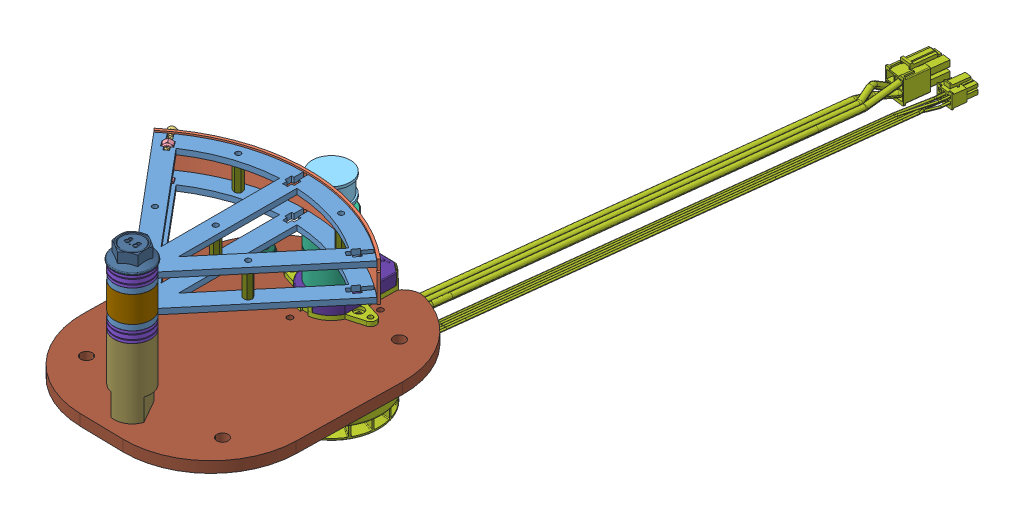
SolidWorks assembly StackedBow, configuration Default. Lengths in mm.
Overall size (130.54 146.72 171.44).
34 component instances, 25 part files, 59 mates.
Components (placement in the parent):
- BowCap-2: BowCap [Default] at origin size (128.56 3.17 110.49)
- BowCap-1: BowCap [Default] at (0 18.2 0) size (128.56 3.17 110.49)
- BowSpacer2-1: BowSpacer2 [Default] at (0 10.9625 76.6044) x (0 0 1) z (-1 0 0) size (24.99 22.7 130.54)
- 91290A053_Black-Oxide Alloy Steel Socket Head Screw-1: 91290A053_Black-Oxide Alloy Steel Socket Head Screw [91290A053] at (-56.2804 20.0625 -0.8589) x (-0.663758 -0.571718 0.482249) z (-0.587785 0 -0.809017) size (4.5 4.5 16.62)
- 94205A101_316 Stainless Steel Nylon-Insert Locknut-3: 94205A101_316 Stainless Steel Nylon-Insert Locknut [94205A101] at (-55.5457 20.0625 0.1523) x (0.809017 0 -0.587785) z (0 -1 0) size (5 3.99 5.77)
- 91290A053_Black-Oxide Alloy Steel Socket Head Screw-2: 91290A053_Black-Oxide Alloy Steel Socket Head Screw [91290A053] at (-56.2804 1.8625 -0.8589) x (-0.545652 -0.738308 0.39644) z (-0.587785 0 -0.809017) size (4.5 4.5 16.62)
- 94205A101_316 Stainless Steel Nylon-Insert Locknut-2: 94205A101_316 Stainless Steel Nylon-Insert Locknut [94205A101] at (-55.5457 1.8625 0.1523) x (0.809017 0 -0.587785) z (0 -1 0) size (5 3.99 5.77)
- Barrel-1: Barrel [Default] at (2.174 4.7125 -35.8745) x (0.993133 0 0.116992) z (-0.116992 0 0.993133) size (22 32.5 22)
- 2469K2_Clamping Shaft Coupling-1: 2469K2_Clamping Shaft Coupling [2469K2] at (2.174 -18.9188 -35.8745) x (0 1 0) z (-0.993133 0 -0.116992) size (35 24 24)
- EC60fl-200W-V2-1: EC60fl-200W-V2 [Default] at (2.174 -29.7 -35.8745) x (0 -1 0) z (-0.993133 0 -0.116992) size (68.19 353.93 60)
- 6655K55_Thrust Ball Bearing-1: 6655K55_Thrust Ball Bearing [6655K55] at (0 -3.175 76.6044) size (21 6.35 21)
- 6655K55_Thrust Ball Bearing-2: 6655K55_Thrust Ball Bearing [6655K55] at (0 24.55 76.6044) size (21 6.35 21)
- BowSpacer3-1: BowSpacer3 [Default] at (0 3.1875 76.6044) size (21 15 21)
- 94036A645_Class 8.8 Steel Flanged Hex Head Screw-1: 94036A645_Class 8.8 Steel Flanged Hex Head Screw [94036A645] at (0 27.725 76.6044) x (1 0 0) z (0 1 0) size (22.3 22.3 54.77)
- Base Plate-1: Base Plate [Default] at (1.2078 -52.8 14.1161) x (-0.019325 0 0.999813) z (-0.999813 0 -0.019325) size (158.6 6.35 125)
- ShaftMount-1: ShaftMount [Default] at (0 -46.45 76.6044) x (0.868119 0 -0.496357) z (0.496357 0 0.868119) size (21 40.1 21)
- 98952A442_Aluminum Male-Female Threaded Hex Standoff-1: 98952A442_Aluminum Male-Female Threaded Hex Standoff [98952A442] at (-37.8185 -68.8 -36.6475) x (0 1 0) z (-0.575536 0 0.817776) size (58.72 15.01 13)
- 91287A207_18-8 Stainless Steel Hex Head Screw-1: 91287A207_18-8 Stainless Steel Hex Head Screw [91287A207] at (-37.8185 -100.8 -36.6475) x (0.849418 0 0.527721) z (0 -1 0) size (10 11.55 18.36)
- 90576A115_Medium-Strength Steel Nylon-Insert Locknut-1: 90576A115_Medium-Strength Steel Nylon-Insert Locknut [90576A115] at (-37.8185 -43.45 -36.6475) x (1 0 0) z (0 1 0) size (10 11.55 6.37)
- 95947A511_Aluminum Female Threaded Hex Standoff-1: 95947A511_Aluminum Female Threaded Hex Standoff [95947A511] at (-26.8742 3.1875 36.7984) x (0 1 0) z (0 0 1) size (15.38 4.5 5.2)
- 95947A511_Aluminum Female Threaded Hex Standoff-2: 95947A511_Aluminum Female Threaded Hex Standoff [95947A511] at (-29.3566 3.1875 -13.7459) x (0 1 0) z (0.188455 0 0.982082) size (15.38 4.5 5.2)
- 95947A511_Aluminum Female Threaded Hex Standoff-3: 95947A511_Aluminum Female Threaded Hex Standoff [95947A511] at (0 3.1875 28.6044) x (0 1 0) z (0.395734 0 0.918365) size (15.38 4.5 5.2)
- 95947A511_Aluminum Female Threaded Hex Standoff-4: 95947A511_Aluminum Female Threaded Hex Standoff [95947A511] at (26.8742 3.1875 36.7984) x (0 1 0) z (0.6 0 0.8) size (15.38 4.5 5.2)
- 95947A511_Aluminum Female Threaded Hex Standoff-5: 95947A511_Aluminum Female Threaded Hex Standoff [95947A511] at (30.1914 3.1875 -13.4704) x (0 1 0) z (0.773678 0 0.63358) size (15.38 4.5 5.2)
- CUI_DEVICES_CUI_DEVICES_AMT102-0048-N8000-W-1: CUI_DEVICES_CUI_DEVICES_AMT102-0048-N8000-W [Default] at (2.174 -42.68 -35.8745) x (-0.999813 0 -0.019325) z (0 1 0) size (52.5 46.23 9.15)
  - CUI_DEVICES_AMT-102-Top-Cover-REV-I-1: CUI_DEVICES_AMT-102-Top-Cover-REV-I [Default] at (0 0 5.23) x (-1 0 0) z (0 0 -1) size (28.6 43.26 6.55)
  - CUI_DEVICES_AMT-Sleeve-REV-D(8 mm)-1: CUI_DEVICES_AMT-Sleeve-REV-D(8 mm) [Default] at (0 0 -2.42) x (0.999996 0.002864 0) z (0 0 1) size (10.79 10.79 7.8)
  - CUI_DEVICES_AMT-Hub-Top-REV-D1-1: CUI_DEVICES_AMT-Hub-Top-REV-D1 [Default] at (0 0 2.13) x (0.999996 0.002864 0) z (0 0 1) size (14 14 5.67)
  - CUI_DEVICES_AMT-Hub-Bottom-REV-B-1: CUI_DEVICES_AMT-Hub-Bottom-REV-B [Default] at (0 0 2.43) x (0.999998 -0.001942 0) z (0 0 1) size (17.3 17.3 3.2)
  - CUI_DEVICES_AMT10X-Shaft-Adaptor-REV-E-1: CUI_DEVICES_AMT10X-Shaft-Adaptor-REV-E [Default] at (0 0 0.03) x (0.999996 0.002864 0) z (0 0 1) size (11.8 11.8 7.8)
  - CUI_DEVICES_Receiver-board-1: CUI_DEVICES_Receiver-board [Default] at (72.2834 -20.351 3.03) x (-1 0 0) z (0 0 -1) size (26.5 26.62 0.41)
  - CUI_DEVICES_Rotor-board-REV F-1: CUI_DEVICES_Rotor-board-REV F [Default] at (0 0 2.13) x (0.807874 -0.589355 0) z (0 0 1) size (26 26 0.3)
  - CUI_DEVICES_Transmitter-board AMT10(AMT-102)-1: CUI_DEVICES_Transmitter-board AMT10(AMT-102) [Default] at (19.1596 -17.1102 1.22) x (-1 0 0) z (0 0 -1) size (26.63 38.43 4.41)
  - CUI_DEVICES_AMT-102-Wide-Base-REV-J-1: CUI_DEVICES_AMT-102-Wide-Base-REV-J [Default] x (-1 0 0) z (0 0 -1) size (52.5 43.41 9.03)
Mates (geometry in assembly coordinates):
- Coincident1: coordinate: point of BowCap-2
- Concentric1: concentric aligned: cylinder of BowCap-2 through (0 3.175 76.6044) axis (0 -1 0) radius 100; cylinder of BowSpacer2-1 through (0 -989.0375 76.6044) axis (0 -1 0) radius 100
- Width1: width aligned: plane of BowSpacer2-1 through (0 10.9625 76.6044) normal (0.766044 0 0.642788); plane of BowSpacer2-1 through (0 10.9625 76.6044) normal (-0.766044 0 0.642788); plane of BowCap-2 through (37.7203 3.175 31.6511) normal (0.766044 0 0.642788); plane of BowCap-2 through (-37.7203 3.175 31.6511) normal (-0.766044 0 0.642788)
- Tangent1: tangent aligned: plane of BowCap-2 through (0 3.175 0) normal (0 1 0); cylinder of BowSpacer2-1 through (-70.8373 1.8625 -20.8947) axis (0.587785 0 0.809017) radius 1.3125
- Concentric2: concentric aligned: cylinder of BowCap-2 through (0 3.175 76.6044) axis (0 -1 0) radius 5; cylinder of BowCap-1 through (0 21.375 76.6044) axis (0 -1 0) radius 5
- Tangent2: tangent aligned: plane of BowCap-1 through (0 21.375 0) normal (0 1 0); cylinder of BowSpacer2-1 through (70.8373 20.0625 -20.8947) axis (-0.587785 0 0.809017) radius 1.3125
- Coincident2: coincident aligned: plane of BowCap-2 through (-37.7203 3.175 31.6511) normal (-0.766044 0 0.642788); plane of BowCap-1 through (-37.7203 21.375 31.6511) normal (-0.766044 0 0.642788)
- Concentric3: concentric aligned: cylinder of BowSpacer2-1 through (-70.8373 20.0625 -20.8947) axis (0.587785 0 0.809017) radius 1.3125; cylinder of 91290A053_Black-Oxide Alloy Steel Socket Head Screw-1 through (-51.4312 20.0625 5.8155) axis (0.587785 0 0.809017) radius 2.25
- Tangent3: tangent anti-aligned: cylinder of BowSpacer2-1 through (0 -989.0375 76.6044) axis (0 -1 0) radius 101.5; plane of 91290A053_Black-Oxide Alloy Steel Socket Head Screw-1 through (-58.2497 21.2774 -6.5356) normal (0.587785 0 0.809017)
- Concentric4: concentric anti-aligned: cylinder of 91290A053_Black-Oxide Alloy Steel Socket Head Screw-1 through (-51.4312 20.0625 5.8155) axis (0.587785 0 0.809017) radius 2.25; cylinder of 94205A101_316 Stainless Steel Nylon-Insert Locknut-3 through (-53.6396 20.0625 2.7759) axis (-0.587785 0 -0.809017) radius 0.9577
- Coincident3: coincident anti-aligned: plane of BowCap-1 through (-55.5457 18.2 0.1523) normal (0.587785 0 0.809017); plane of 94205A101_316 Stainless Steel Nylon-Insert Locknut-3 through (-53.5232 21.5059 -1.3171) normal (-0.587785 0 -0.809017)
- Parallel1: parallel anti-aligned: plane of BowCap-1 through (-47.2518 18.2 16.2466) normal (0.809017 0 -0.587785); plane of 94205A101_316 Stainless Steel Nylon-Insert Locknut-3 through (-55.3347 21.5059 4.6961) normal (-0.809017 0 0.587785)
- Concentric5: concentric anti-aligned: cylinder of 91290A053_Black-Oxide Alloy Steel Socket Head Screw-2 through (-51.4312 1.8625 5.8155) axis (0.587785 0 0.809017) radius 2.25; cylinder of 94205A101_316 Stainless Steel Nylon-Insert Locknut-2 through (-53.6396 1.8625 2.7759) axis (-0.587785 0 -0.809017) radius 0.9577
- Concentric6: concentric aligned: cylinder of BowSpacer2-1 through (-70.8373 1.8625 -20.8947) axis (0.587785 0 0.809017) radius 1.3125; cylinder of 91290A053_Black-Oxide Alloy Steel Socket Head Screw-2 through (-51.4312 1.8625 5.8155) axis (0.587785 0 0.809017) radius 2.25
- Tangent4: tangent anti-aligned: cylinder of BowSpacer2-1 through (0 -989.0375 76.6044) axis (0 -1 0) radius 101.5; plane of 91290A053_Black-Oxide Alloy Steel Socket Head Screw-2 through (-58.5007 3.4314 -6.3532) normal (0.587785 0 0.809017)
- Coincident5: coincident anti-aligned: plane of BowCap-2 through (-55.5457 0 0.1523) normal (0.587785 0 0.809017); plane of 94205A101_316 Stainless Steel Nylon-Insert Locknut-2 through (-53.5232 3.3059 -1.3171) normal (-0.587785 0 -0.809017)
- Parallel2: parallel anti-aligned: plane of BowCap-2 through (-47.2518 0 16.2466) normal (0.809017 0 -0.587785); plane of 94205A101_316 Stainless Steel Nylon-Insert Locknut-2 through (-55.3347 3.3059 4.6961) normal (-0.809017 0 0.587785)
- Width2: width aligned: plane of Barrel-1 through (-8.7504 17.2125 -37.1615) normal (0 1 0); plane of Barrel-1 through (-1.7985 4.7125 -36.3425) normal (0 -1 0); plane of BowSpacer2-1 through (-65.2429 22.3125 -1.1491) normal (0 1 0); plane of BowSpacer2-1 through (-65.2429 -0.3875 -1.1491) normal (0 -1 0)
- Tangent7: tangent anti-aligned: cylinder of BowSpacer2-1 through (0 -989.0375 76.6044) axis (0 -1 0) radius 101.5; cylinder of Barrel-1 through (2.174 17.2125 -35.8745) axis (0 1 0) radius 11
- Concentric7: concentric anti-aligned: cylinder of Barrel-1 through (2.174 17.2125 -35.8745) axis (0 1 0) radius 4; cylinder of 2469K2_Clamping Shaft Coupling-1 through (2.174 -36.4188 -35.8745) axis (0 -1 0) radius 4
- Concentric8: concentric aligned: cylinder of 2469K2_Clamping Shaft Coupling-1 through (2.174 -36.4188 -35.8745) axis (0 -1 0) radius 4; cylinder of EC60fl-200W-V2-1 through (2.174 -26.635 -35.8745) axis (0 -1 0) radius 4
- Coincident8: coincident aligned: plane of Barrel-1 through (2.174 4.7125 -35.8745) normal (-0.116992 0 0.993133); plane of EC60fl-200W-V2-1 through (2.174 -29.7 -35.8745) normal (-0.116992 0 0.993133)
- Coincident9: coincident anti-aligned: plane of 2469K2_Clamping Shaft Coupling-1 through (2.174 -18.9188 -35.8745) normal (0.116992 0 -0.993133); plane of EC60fl-200W-V2-1 through (2.174 -29.7 -35.8745) normal (-0.116992 0 0.993133)
- Distance4: distance = 11 mm: plane of Barrel-1 through (2.174 4.7125 -35.8745) normal (0.993133 0 0.116992); cylinder of BowSpacer2-1 through (0 -989.0375 76.6044) axis (0 -1 0) radius 101.5
- Coincident10: coincident anti-aligned: plane of BowCap-2 through (0 0 0) normal (0 -1 0); plane of 6655K55_Thrust Ball Bearing-1 through (10.5 0 76.6044) normal (0 1 0)
- Concentric9: concentric anti-aligned: cylinder of BowCap-2 through (0 3.175 76.6044) axis (0 -1 0) radius 5; cylinder of 6655K55_Thrust Ball Bearing-1 through (0 0 76.6044) axis (0 1 0) radius 5
- Concentric10: concentric anti-aligned: cylinder of BowCap-1 through (0 21.375 76.6044) axis (0 -1 0) radius 5; cylinder of 6655K55_Thrust Ball Bearing-2 through (0 27.725 76.6044) axis (0 1 0) radius 5
- Coincident11: coincident anti-aligned: plane of BowCap-1 through (0 21.375 0) normal (0 1 0); plane of 6655K55_Thrust Ball Bearing-2 through (10.5 21.375 76.6044) normal (0 -1 0)
- Concentric11: concentric aligned: cylinder of BowCap-2 through (0 3.175 76.6044) axis (0 -1 0) radius 5; cylinder of BowSpacer3-1 through (0 18.1875 76.6044) axis (0 -1 0) radius 5.5
- Width6: width anti-aligned: plane of BowCap-2 through (0 3.175 0) normal (0 1 0); plane of BowCap-1 through (0 18.2 0) normal (0 -1 0); plane of BowSpacer3-1 through (0 3.1875 76.6044) normal (0 -1 0); plane of BowSpacer3-1 through (0 18.1875 76.6044) normal (0 1 0)
- Concentric12: concentric anti-aligned: cylinder of BowCap-1 through (0 21.375 76.6044) axis (0 -1 0) radius 5; cylinder of 94036A645_Class 8.8 Steel Flanged Hex Head Screw-1 through (0 -17.275 76.6044) axis (0 1 0) radius 5
- Coincident12: coincident anti-aligned: plane of 6655K55_Thrust Ball Bearing-2 through (10.5 27.725 76.6044) normal (0 1 0); plane of 94036A645_Class 8.8 Steel Flanged Hex Head Screw-1 through (-7.5 27.725 89.5948) normal (0 -1 0)
- Coincident13: coincident anti-aligned: plane of EC60fl-200W-V2-1 through (2.174 -52.8 -35.8745) normal (0 1 0); plane of Base Plate-1 through (1.2078 -52.8 14.1161) normal (0 -1 0)
- Coincident14: coincident aligned: point of EC60fl-200W-V2-1; plane of Base Plate-1 through (1.2078 -52.8 14.1161) normal (-0.999813 0 -0.019325)
- Distance5: distance = 130 mm: plane of Base Plate-1 through (-0.3382 -46.45 94.1012) normal (-0.019325 0 0.999813); point of EC60fl-200W-V2-1
- Coincident15: coincident anti-aligned: plane of 6655K55_Thrust Ball Bearing-1 through (10.5 -6.35 76.6044) normal (0 -1 0); plane of ShaftMount-1 through (0 -6.35 76.6044) normal (0 1 0)
- Concentric13: concentric anti-aligned: cylinder of BowCap-2 through (0 3.175 76.6044) axis (0 -1 0) radius 10.5; cylinder of ShaftMount-1 through (0 -6.35 76.6044) axis (0 1 0) radius 4.5
- Coincident26: coincident anti-aligned: plane of Base Plate-1 through (1.2078 -52.8 14.1161) normal (-0.999813 0 -0.019325); point of ShaftMount-1
- Concentric15: concentric anti-aligned: cylinder of Base Plate-1 through (-37.8185 -46.45 -36.6475) axis (0 1 0) radius 3.3; circle of 98952A442_Aluminum Male-Female Threaded Hex Standoff-1
- Coincident22: coincident anti-aligned: plane of Base Plate-1 through (1.2078 -52.8 14.1161) normal (0 -1 0); plane of 98952A442_Aluminum Male-Female Threaded Hex Standoff-1 through (-43.9564 -52.8 -40.9673) normal (0 1 0)
- Concentric16: concentric aligned: circle of 98952A442_Aluminum Male-Female Threaded Hex Standoff-1; circle of 91287A207_18-8 Stainless Steel Hex Head Screw-1
- Distance7: distance = 8 mm anti-aligned: plane of 98952A442_Aluminum Male-Female Threaded Hex Standoff-1 through (-43.9564 -97.8 -40.9673) normal (0 -1 0); plane of 91287A207_18-8 Stainless Steel Hex Head Screw-1 through (-40.8653 -105.8 -31.7434) normal (0 1 0)
- Concentric17: concentric anti-aligned: circle of 98952A442_Aluminum Male-Female Threaded Hex Standoff-1; cylinder of 90576A115_Medium-Strength Steel Nylon-Insert Locknut-1 through (-37.8185 -46.45 -36.6475) axis (0 -1 0) radius 2.3505
- Coincident24: coincident anti-aligned: plane of Base Plate-1 through (1.2078 -46.45 14.1161) normal (0 1 0); plane of 90576A115_Medium-Strength Steel Nylon-Insert Locknut-1 through (-37.8185 -46.45 -36.6475) normal (0 -1 0)
- Width7: width anti-aligned: plane of 2469K2_Clamping Shaft Coupling-1 through (14.0916 -1.4188 -34.4706) normal (0 1 0); plane of 2469K2_Clamping Shaft Coupling-1 through (6.1466 -36.4188 -35.4066) normal (0 -1 0); plane of BowSpacer2-1 through (-65.2429 -0.3875 -1.1491) normal (0 -1 0); plane of CUI_DEVICES_CUI_DEVICES_AMT102-0048-N8000-W-1/CUI_DEVICES_AMT-102-Top-Cover-REV-I-1 through (2.174 -37.45 -35.8745) normal (0 1 0)
- Coincident25: coincident anti-aligned: plane of Base Plate-1 through (1.2078 -46.45 14.1161) normal (0 1 0); plane of ShaftMount-1 through (0 -46.45 76.6044) normal (0 -1 0)
- Width8: width anti-aligned: plane of BowCap-2 through (0 3.175 0) normal (0 1 0); plane of 95947A511_Aluminum Female Threaded Hex Standoff-1 through (0 18.2 0) normal (0 -1 0); plane of BowCap-1 through (-26.8742 3.1875 36.7984) normal (0 -1 0); plane of 95947A511_Aluminum Female Threaded Hex Standoff-1 through (-26.8742 18.1875 36.7984) normal (0 1 0)
- Concentric18: concentric anti-aligned: cylinder of BowCap-2 through (-26.8742 3.175 36.7984) axis (0 1 0) radius 1.5; circle of 95947A511_Aluminum Female Threaded Hex Standoff-1
- Width9: width anti-aligned: plane of BowCap-2 through (0 3.175 0) normal (0 1 0); plane of 95947A511_Aluminum Female Threaded Hex Standoff-2 through (0 18.2 0) normal (0 -1 0); plane of BowCap-1 through (-29.3566 3.1875 -13.7459) normal (0 -1 0); plane of 95947A511_Aluminum Female Threaded Hex Standoff-2 through (-29.3566 18.1875 -13.7459) normal (0 1 0)
- Concentric19: concentric anti-aligned: cylinder of BowCap-2 through (-29.3566 3.175 -13.7459) axis (0 1 0) radius 1.5; circle of 95947A511_Aluminum Female Threaded Hex Standoff-2
- Width10: width anti-aligned: plane of BowCap-2 through (0 3.175 0) normal (0 1 0); plane of 95947A511_Aluminum Female Threaded Hex Standoff-3 through (0 18.2 0) normal (0 -1 0); plane of BowCap-1 through (0 3.1875 28.6044) normal (0 -1 0); plane of 95947A511_Aluminum Female Threaded Hex Standoff-3 through (0 18.1875 28.6044) normal (0 1 0)
- Concentric20: concentric anti-aligned: cylinder of BowCap-2 through (0 3.175 28.6044) axis (0 1 0) radius 1.5; circle of 95947A511_Aluminum Female Threaded Hex Standoff-3
- Width11: width anti-aligned: plane of BowCap-2 through (0 3.175 0) normal (0 1 0); plane of 95947A511_Aluminum Female Threaded Hex Standoff-4 through (0 18.2 0) normal (0 -1 0); plane of BowCap-1 through (26.8742 3.1875 36.7984) normal (0 -1 0); plane of 95947A511_Aluminum Female Threaded Hex Standoff-4 through (26.8742 18.1875 36.7984) normal (0 1 0)
- Concentric21: concentric anti-aligned: cylinder of BowCap-2 through (26.8742 3.175 36.7984) axis (0 1 0) radius 1.5; circle of 95947A511_Aluminum Female Threaded Hex Standoff-4
- Width12: width anti-aligned: plane of BowCap-2 through (0 3.175 0) normal (0 1 0); plane of 95947A511_Aluminum Female Threaded Hex Standoff-5 through (0 18.2 0) normal (0 -1 0); plane of BowCap-1 through (30.1914 3.1875 -13.4704) normal (0 -1 0); plane of 95947A511_Aluminum Female Threaded Hex Standoff-5 through (30.1914 18.1875 -13.4704) normal (0 1 0)
- Concentric22: concentric anti-aligned: cylinder of BowCap-2 through (30.1914 3.175 -13.4704) axis (0 1 0) radius 1.5; circle of 95947A511_Aluminum Female Threaded Hex Standoff-5
- Coincident27: coincident anti-aligned: plane of Base Plate-1 through (1.2078 -46.45 14.1161) normal (0 1 0); plane of CUI_DEVICES_CUI_DEVICES_AMT102-0048-N8000-W-1/CUI_DEVICES_AMT-102-Wide-Base-REV-J-1 through (2.3754 -46.45 -46.2926) normal (0 -1 0)
- Concentric23: concentric anti-aligned: cylinder of EC60fl-200W-V2-1 through (2.174 -26.635 -35.8745) axis (0 -1 0) radius 4; cylinder of CUI_DEVICES_CUI_DEVICES_AMT102-0048-N8000-W-1/CUI_DEVICES_AMT-102-Top-Cover-REV-I-1 through (2.174 -43.95 -35.8745) axis (0 1 0) radius 7.65
- Parallel3: parallel aligned: plane of Base Plate-1 through (1.2078 -52.8 14.1161) normal (-0.999813 0 -0.019325); plane of CUI_DEVICES_CUI_DEVICES_AMT102-0048-N8000-W-1 through (2.174 -42.68 -35.8745) normal (-0.999813 0 -0.019325)
